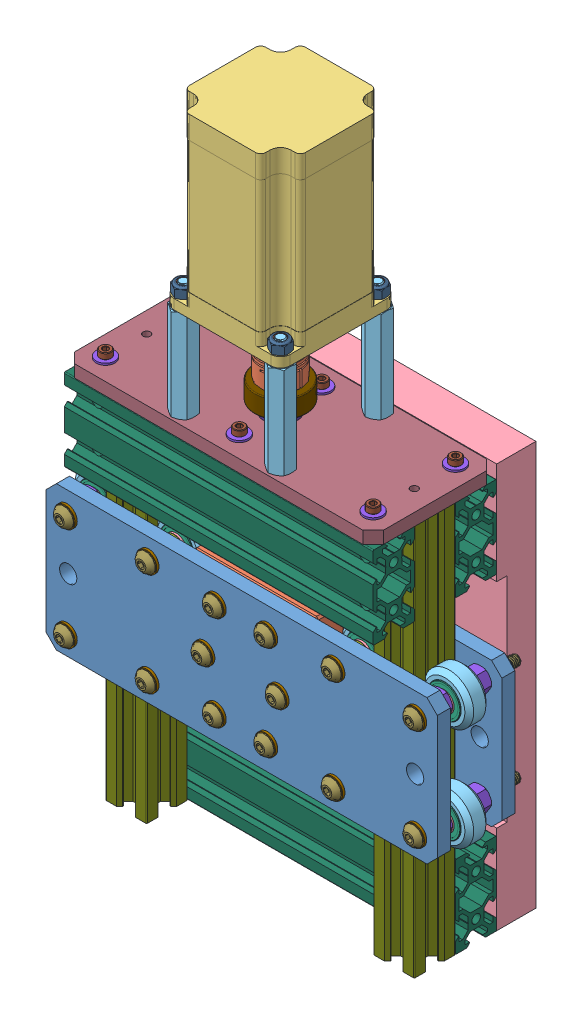
SolidWorks assembly Longitudinal Trim Assembly, configuration Default. Lengths in mm. (continued)
Components (placement in the parent): (continued)
- 91100A120 - WASHER, M3 X 9 OD, 18-8-2: 91100A120 - WASHER, M3 X 9 OD, 18-8 [93475A210] at (65 -65 17.3) x (0.993328 0.115328 0) z (0 0 1) size (9 9 0.9)
- 94500A222 - BHCS, M3-0.5 X 8, 316 SS-2: 94500A222 - BHCS, M3-0.5 X 8, 316 SS [94500A222] at (65 -65 15.65) x (-0.923728 -0.383049 0) z (0 0 -1) size (5.7 5.7 9.95)
- HNTTBS5-3 - NUT, PRE-INSERTION, M3 X 10 SQ, 18-8-3: HNTTBS5-3 - NUT, PRE-INSERTION, M3 X 10 SQ, 18-8 [Default] at (65 65 21.8) x (0 0 -1) z (0 -1 0) size (2.7 10 10)
- 91100A120 - WASHER, M3 X 9 OD, 18-8-3: 91100A120 - WASHER, M3 X 9 OD, 18-8 [93475A210] at (65 65 17.3) x (0.993328 0.115328 0) z (0 0 1) size (9 9 0.9)
- 94500A222 - BHCS, M3-0.5 X 8, 316 SS-3: 94500A222 - BHCS, M3-0.5 X 8, 316 SS [94500A222] at (65 65 15.65) x (-0.923728 -0.383049 0) z (0 0 -1) size (5.7 5.7 9.95)
- HNTTBS5-3 - NUT, PRE-INSERTION, M3 X 10 SQ, 18-8-4: HNTTBS5-3 - NUT, PRE-INSERTION, M3 X 10 SQ, 18-8 [Default] at (65 85 21.8) x (0 0 -1) z (0 -1 0) size (2.7 10 10)
- 91100A120 - WASHER, M3 X 9 OD, 18-8-4: 91100A120 - WASHER, M3 X 9 OD, 18-8 [93475A210] at (65 85 17.3) x (0.993328 0.115328 0) z (0 0 1) size (9 9 0.9)
- 94500A222 - BHCS, M3-0.5 X 8, 316 SS-4: 94500A222 - BHCS, M3-0.5 X 8, 316 SS [94500A222] at (65 85 15.65) x (-0.923728 -0.383049 0) z (0 0 -1) size (5.7 5.7 9.95)
- HNTTBS5-3 - NUT, PRE-INSERTION, M3 X 10 SQ, 18-8-5: HNTTBS5-3 - NUT, PRE-INSERTION, M3 X 10 SQ, 18-8 [Default] at (65 65 38.2) x (0 0 -1) z (0 -1 0) size (2.7 10 10)
- 91100A120 - WASHER, M3 X 9 OD, 18-8-5: 91100A120 - WASHER, M3 X 9 OD, 18-8 [93475A210] at (65 65 42.7) x (0.961741 0.273962 0) z (0 0 -1) size (9 9 0.9)
- 94500A222 - BHCS, M3-0.5 X 8, 316 SS-5: 94500A222 - BHCS, M3-0.5 X 8, 316 SS [94500A222] at (65 65 44.35) x (-0.923728 -0.383049 0) z (0 0 1) size (5.7 5.7 9.95)
- HNTTBS5-3 - NUT, PRE-INSERTION, M3 X 10 SQ, 18-8-6: HNTTBS5-3 - NUT, PRE-INSERTION, M3 X 10 SQ, 18-8 [Default] at (65 85 38.2) x (0 0 -1) z (0 -1 0) size (2.7 10 10)
- 91100A120 - WASHER, M3 X 9 OD, 18-8-6: 91100A120 - WASHER, M3 X 9 OD, 18-8 [93475A210] at (65 85 42.7) x (0.961741 0.273962 0) z (0 0 -1) size (9 9 0.9)
- 94500A222 - BHCS, M3-0.5 X 8, 316 SS-6: 94500A222 - BHCS, M3-0.5 X 8, 316 SS [94500A222] at (65 85 44.35) x (-1 0 0) z (0 0 1) size (5.7 5.7 9.95)
- HNTTBS5-3 - NUT, PRE-INSERTION, M3 X 10 SQ, 18-8-9: HNTTBS5-3 - NUT, PRE-INSERTION, M3 X 10 SQ, 18-8 [Default] at (-65 85 1.8) x (0 0 -1) z (1 0 0) size (2.7 10 10)
- 91420A130 - FHS, 90 DEG, M3-0.5 X 25, STEEL, ZINC-13: 91420A130 - FHS, 90 DEG, M3-0.5 X 25, STEEL, ZINC [91420A130] at (-65 85 -17.05) x (-0.923728 -0.383049 0) z (0 0 -1) size (5.6 5.6 25.28)
- HNTTBS5-3 - NUT, PRE-INSERTION, M3 X 10 SQ, 18-8-29: HNTTBS5-3 - NUT, PRE-INSERTION, M3 X 10 SQ, 18-8 [Default] at (65 93.2 50) x (0 1 0) z (1 0 0) size (2.7 10 10)
- 91100A120 - WASHER, M3 X 9 OD, 18-8-14: 91100A120 - WASHER, M3 X 9 OD, 18-8 [93475A210] at (65 101 50) x (0.993663 0 -0.112402) z (0 1 0) size (9 9 0.9)
- 91292A114 - SHCS, M3-0.5 X 12, 18-8-1: 91292A114 - SHCS, M3-0.5 X 12, 18-8 [91292A114] at (65 89.9 50) x (-0.862717 0 -0.505687) z (0 -1 0) size (5.5 5.5 15.23)
- HNTTBS5-3 - NUT, PRE-INSERTION, M3 X 10 SQ, 18-8-12: HNTTBS5-3 - NUT, PRE-INSERTION, M3 X 10 SQ, 18-8 [Default] at (0 -85 1.8) x (0 0 -1) z (1 0 0) size (2.7 10 10)
- HNTTBS5-3 - NUT, PRE-INSERTION, M3 X 10 SQ, 18-8-13: HNTTBS5-3 - NUT, PRE-INSERTION, M3 X 10 SQ, 18-8 [Default] at (0 -65 1.8) x (0 0 -1) z (1 0 0) size (2.7 10 10)
- HNTTBS5-3 - NUT, PRE-INSERTION, M3 X 10 SQ, 18-8-14: HNTTBS5-3 - NUT, PRE-INSERTION, M3 X 10 SQ, 18-8 [Default] at (0 65 1.8) x (0 0 -1) z (1 0 0) size (2.7 10 10)
- HNTTBS5-3 - NUT, PRE-INSERTION, M3 X 10 SQ, 18-8-15: HNTTBS5-3 - NUT, PRE-INSERTION, M3 X 10 SQ, 18-8 [Default] at (0 85 1.8) x (0 0 -1) z (1 0 0) size (2.7 10 10)
- HNTTBS5-3 - NUT, PRE-INSERTION, M3 X 10 SQ, 18-8-16: HNTTBS5-3 - NUT, PRE-INSERTION, M3 X 10 SQ, 18-8 [Default] at (-65 -85 1.8) x (0 0 -1) z (1 0 0) size (2.7 10 10)
- HNTTBS5-3 - NUT, PRE-INSERTION, M3 X 10 SQ, 18-8-17: HNTTBS5-3 - NUT, PRE-INSERTION, M3 X 10 SQ, 18-8 [Default] at (-65 -65 1.8) x (0 0 -1) z (1 0 0) size (2.7 10 10)
- HNTTBS5-3 - NUT, PRE-INSERTION, M3 X 10 SQ, 18-8-18: HNTTBS5-3 - NUT, PRE-INSERTION, M3 X 10 SQ, 18-8 [Default] at (65 -85 1.8) x (0 0 -1) z (1 0 0) size (2.7 10 10)
- HNTTBS5-3 - NUT, PRE-INSERTION, M3 X 10 SQ, 18-8-19: HNTTBS5-3 - NUT, PRE-INSERTION, M3 X 10 SQ, 18-8 [Default] at (-65 65 1.8) x (0 0 -1) z (1 0 0) size (2.7 10 10)
- HNTTBS5-3 - NUT, PRE-INSERTION, M3 X 10 SQ, 18-8-20: HNTTBS5-3 - NUT, PRE-INSERTION, M3 X 10 SQ, 18-8 [Default] at (65 65 1.8) x (0 0 -1) z (1 0 0) size (2.7 10 10)
- HNTTBS5-3 - NUT, PRE-INSERTION, M3 X 10 SQ, 18-8-21: HNTTBS5-3 - NUT, PRE-INSERTION, M3 X 10 SQ, 18-8 [Default] at (65 85 1.8) x (0 0 -1) z (1 0 0) size (2.7 10 10)
- HNTTBS5-3 - NUT, PRE-INSERTION, M3 X 10 SQ, 18-8-22: HNTTBS5-3 - NUT, PRE-INSERTION, M3 X 10 SQ, 18-8 [Default] at (65 -65 1.8) x (0 0 -1) z (1 0 0) size (2.7 10 10)
- 91420A130 - FHS, 90 DEG, M3-0.5 X 25, STEEL, ZINC-14: 91420A130 - FHS, 90 DEG, M3-0.5 X 25, STEEL, ZINC [91420A130] at (0 -85 -17.05) x (-0.923728 -0.383049 0) z (0 0 -1) size (5.6 5.6 25.28)
- 91420A130 - FHS, 90 DEG, M3-0.5 X 25, STEEL, ZINC-15: 91420A130 - FHS, 90 DEG, M3-0.5 X 25, STEEL, ZINC [91420A130] at (0 -65 -17.05) x (-0.923728 -0.383049 0) z (0 0 -1) size (5.6 5.6 25.28)
- 91420A130 - FHS, 90 DEG, M3-0.5 X 25, STEEL, ZINC-16: 91420A130 - FHS, 90 DEG, M3-0.5 X 25, STEEL, ZINC [91420A130] at (0 65 -17.05) x (-0.923728 -0.383049 0) z (0 0 -1) size (5.6 5.6 25.28)
- 91420A130 - FHS, 90 DEG, M3-0.5 X 25, STEEL, ZINC-17: 91420A130 - FHS, 90 DEG, M3-0.5 X 25, STEEL, ZINC [91420A130] at (0 85 -17.05) x (-0.923728 -0.383049 0) z (0 0 -1) size (5.6 5.6 25.28)
- 91420A130 - FHS, 90 DEG, M3-0.5 X 25, STEEL, ZINC-18: 91420A130 - FHS, 90 DEG, M3-0.5 X 25, STEEL, ZINC [91420A130] at (-65 -85 -17.05) x (-0.923728 -0.383049 0) z (0 0 -1) size (5.6 5.6 25.28)
- 91420A130 - FHS, 90 DEG, M3-0.5 X 25, STEEL, ZINC-19: 91420A130 - FHS, 90 DEG, M3-0.5 X 25, STEEL, ZINC [91420A130] at (-65 -65 -17.05) x (-0.923728 -0.383049 0) z (0 0 -1) size (5.6 5.6 25.28)
- 91420A130 - FHS, 90 DEG, M3-0.5 X 25, STEEL, ZINC-20: 91420A130 - FHS, 90 DEG, M3-0.5 X 25, STEEL, ZINC [91420A130] at (65 -85 -17.05) x (-0.923728 -0.383049 0) z (0 0 -1) size (5.6 5.6 25.28)
- 91420A130 - FHS, 90 DEG, M3-0.5 X 25, STEEL, ZINC-21: 91420A130 - FHS, 90 DEG, M3-0.5 X 25, STEEL, ZINC [91420A130] at (-65 65 -17.05) x (-0.923728 -0.383049 0) z (0 0 -1) size (5.6 5.6 25.28)
- 91420A130 - FHS, 90 DEG, M3-0.5 X 25, STEEL, ZINC-22: 91420A130 - FHS, 90 DEG, M3-0.5 X 25, STEEL, ZINC [91420A130] at (65 65 -17.05) x (-0.923728 -0.383049 0) z (0 0 -1) size (5.6 5.6 25.28)
- 91420A130 - FHS, 90 DEG, M3-0.5 X 25, STEEL, ZINC-23: 91420A130 - FHS, 90 DEG, M3-0.5 X 25, STEEL, ZINC [91420A130] at (65 85 -17.05) x (-0.923728 -0.383049 0) z (0 0 -1) size (5.6 5.6 25.28)
- 91420A130 - FHS, 90 DEG, M3-0.5 X 25, STEEL, ZINC-24: 91420A130 - FHS, 90 DEG, M3-0.5 X 25, STEEL, ZINC [91420A130] at (65 -65 -17.05) x (-0.923728 -0.383049 0) z (0 0 -1) size (5.6 5.6 25.28)
- HNTTBS5-3 - NUT, PRE-INSERTION, M3 X 10 SQ, 18-8-23: HNTTBS5-3 - NUT, PRE-INSERTION, M3 X 10 SQ, 18-8 [Default] at (-65 -85 21.8) x (0 0 -1) z (0 1 0) size (2.7 10 10)
- 91100A120 - WASHER, M3 X 9 OD, 18-8-8: 91100A120 - WASHER, M3 X 9 OD, 18-8 [93475A210] at (-65 -85 18.2) x (-0.993328 0.115328 0) z (0 0 -1) size (9 9 0.9)
- 94500A222 - BHCS, M3-0.5 X 8, 316 SS-8: 94500A222 - BHCS, M3-0.5 X 8, 316 SS [94500A222] at (-65 -85 15.65) x (0.923728 -0.383049 0) z (0 0 -1) size (5.7 5.7 9.95)
- HNTTBS5-3 - NUT, PRE-INSERTION, M3 X 10 SQ, 18-8-24: HNTTBS5-3 - NUT, PRE-INSERTION, M3 X 10 SQ, 18-8 [Default] at (-65 -65 21.8) x (0 0 -1) z (0 1 0) size (2.7 10 10)
- 91100A120 - WASHER, M3 X 9 OD, 18-8-9: 91100A120 - WASHER, M3 X 9 OD, 18-8 [93475A210] at (-65 -65 18.2) x (-0.993328 0.115328 0) z (0 0 -1) size (9 9 0.9)
- 94500A222 - BHCS, M3-0.5 X 8, 316 SS-9: 94500A222 - BHCS, M3-0.5 X 8, 316 SS [94500A222] at (-65 -65 15.65) x (0.923728 -0.383049 0) z (0 0 -1) size (5.7 5.7 9.95)
- HNTTBS5-3 - NUT, PRE-INSERTION, M3 X 10 SQ, 18-8-25: HNTTBS5-3 - NUT, PRE-INSERTION, M3 X 10 SQ, 18-8 [Default] at (-65 65 21.8) x (0 0 -1) z (0 1 0) size (2.7 10 10)
- 91100A120 - WASHER, M3 X 9 OD, 18-8-10: 91100A120 - WASHER, M3 X 9 OD, 18-8 [93475A210] at (-65 65 18.2) x (-0.993328 0.115328 0) z (0 0 -1) size (9 9 0.9)
- 94500A222 - BHCS, M3-0.5 X 8, 316 SS-10: 94500A222 - BHCS, M3-0.5 X 8, 316 SS [94500A222] at (-65 65 15.65) x (0.923728 -0.383049 0) z (0 0 -1) size (5.7 5.7 9.95)
- HNTTBS5-3 - NUT, PRE-INSERTION, M3 X 10 SQ, 18-8-26: HNTTBS5-3 - NUT, PRE-INSERTION, M3 X 10 SQ, 18-8 [Default] at (-65 85 21.8) x (0 0 -1) z (0 1 0) size (2.7 10 10)
- 91100A120 - WASHER, M3 X 9 OD, 18-8-11: 91100A120 - WASHER, M3 X 9 OD, 18-8 [93475A210] at (-65 85 18.2) x (-0.993328 0.115328 0) z (0 0 -1) size (9 9 0.9)
- 94500A222 - BHCS, M3-0.5 X 8, 316 SS-11: 94500A222 - BHCS, M3-0.5 X 8, 316 SS [94500A222] at (-65 85 15.65) x (0.923728 -0.383049 0) z (0 0 -1) size (5.7 5.7 9.95)
- HNTTBS5-3 - NUT, PRE-INSERTION, M3 X 10 SQ, 18-8-27: HNTTBS5-3 - NUT, PRE-INSERTION, M3 X 10 SQ, 18-8 [Default] at (-65 65 38.2) x (0 0 -1) z (0 1 0) size (2.7 10 10)
- 91100A120 - WASHER, M3 X 9 OD, 18-8-12: 91100A120 - WASHER, M3 X 9 OD, 18-8 [93475A210] at (-65 65 41.8) x (-0.961741 0.273962 0) z (0 0 1) size (9 9 0.9)
- 94500A222 - BHCS, M3-0.5 X 8, 316 SS-12: 94500A222 - BHCS, M3-0.5 X 8, 316 SS [94500A222] at (-65 65 44.35) x (0.923728 -0.383049 0) z (0 0 1) size (5.7 5.7 9.95)
- HNTTBS5-3 - NUT, PRE-INSERTION, M3 X 10 SQ, 18-8-28: HNTTBS5-3 - NUT, PRE-INSERTION, M3 X 10 SQ, 18-8 [Default] at (-65 85 38.2) x (0 0 -1) z (0 1 0) size (2.7 10 10)
- 91100A120 - WASHER, M3 X 9 OD, 18-8-13: 91100A120 - WASHER, M3 X 9 OD, 18-8 [93475A210] at (-65 85 41.8) x (-0.961741 0.273962 0) z (0 0 1) size (9 9 0.9)
- 94500A222 - BHCS, M3-0.5 X 8, 316 SS-13: 94500A222 - BHCS, M3-0.5 X 8, 316 SS [94500A222] at (-65 85 44.35) size (5.7 5.7 9.95)
- HNTTBS5-3 - NUT, PRE-INSERTION, M3 X 10 SQ, 18-8-31: HNTTBS5-3 - NUT, PRE-INSERTION, M3 X 10 SQ, 18-8 [Default] at (-65 93.2 10) x (0 1 0) z (1 0 0) size (2.7 10 10)
- HNTTBS5-3 - NUT, PRE-INSERTION, M3 X 10 SQ, 18-8-32: HNTTBS5-3 - NUT, PRE-INSERTION, M3 X 10 SQ, 18-8 [Default] at (65 93.2 10) x (0 1 0) z (1 0 0) size (2.7 10 10)
- HNTTBS5-3 - NUT, PRE-INSERTION, M3 X 10 SQ, 18-8-33: HNTTBS5-3 - NUT, PRE-INSERTION, M3 X 10 SQ, 18-8 [Default] at (0 93.2 50) x (0 1 0) z (1 0 0) size (2.7 10 10)
- HNTTBS5-3 - NUT, PRE-INSERTION, M3 X 10 SQ, 18-8-34: HNTTBS5-3 - NUT, PRE-INSERTION, M3 X 10 SQ, 18-8 [Default] at (0 93.2 10) x (0 1 0) z (1 0 0) size (2.7 10 10)
- HNTTBS5-3 - NUT, PRE-INSERTION, M3 X 10 SQ, 18-8-35: HNTTBS5-3 - NUT, PRE-INSERTION, M3 X 10 SQ, 18-8 [Default] at (-65 93.2 50) x (0 1 0) z (1 0 0) size (2.7 10 10)
- 91100A120 - WASHER, M3 X 9 OD, 18-8-15: 91100A120 - WASHER, M3 X 9 OD, 18-8 [93475A210] at (-65 101 10) x (0.993663 0 -0.112402) z (0 1 0) size (9 9 0.9)
- 91100A120 - WASHER, M3 X 9 OD, 18-8-16: 91100A120 - WASHER, M3 X 9 OD, 18-8 [93475A210] at (65 101 10) x (0.993663 0 -0.112402) z (0 1 0) size (9 9 0.9)
- 91100A120 - WASHER, M3 X 9 OD, 18-8-17: 91100A120 - WASHER, M3 X 9 OD, 18-8 [93475A210] at (0 101 50) x (0.993663 0 -0.112402) z (0 1 0) size (9 9 0.9)
- 91100A120 - WASHER, M3 X 9 OD, 18-8-18: 91100A120 - WASHER, M3 X 9 OD, 18-8 [93475A210] at (0 101 10) x (0.993663 0 -0.112402) z (0 1 0) size (9 9 0.9)
- 91100A120 - WASHER, M3 X 9 OD, 18-8-19: 91100A120 - WASHER, M3 X 9 OD, 18-8 [93475A210] at (-65 101 50) x (0.993663 0 -0.112402) z (0 1 0) size (9 9 0.9)
- 91292A114 - SHCS, M3-0.5 X 12, 18-8-2: 91292A114 - SHCS, M3-0.5 X 12, 18-8 [91292A114] at (-65 89.9 10) x (-0.862717 0 -0.505687) z (0 -1 0) size (5.5 5.5 15.23)
- 91292A114 - SHCS, M3-0.5 X 12, 18-8-3: 91292A114 - SHCS, M3-0.5 X 12, 18-8 [91292A114] at (65 89.9 10) x (-0.862717 0 -0.505687) z (0 -1 0) size (5.5 5.5 15.23)
- 91292A114 - SHCS, M3-0.5 X 12, 18-8-4: 91292A114 - SHCS, M3-0.5 X 12, 18-8 [91292A114] at (0 89.9 50) x (-0.862717 0 -0.505687) z (0 -1 0) size (5.5 5.5 15.23)
- 91292A114 - SHCS, M3-0.5 X 12, 18-8-5: 91292A114 - SHCS, M3-0.5 X 12, 18-8 [91292A114] at (0 89.9 10) x (-0.862717 0 -0.505687) z (0 -1 0) size (5.5 5.5 15.23)
- 91292A114 - SHCS, M3-0.5 X 12, 18-8-6: 91292A114 - SHCS, M3-0.5 X 12, 18-8 [91292A114] at (-65 89.9 50) x (-0.862717 0 -0.505687) z (0 -1 0) size (5.5 5.5 15.23)
Mates (geometry in assembly coordinates):
- Concentric56: concentric aligned: cylinder of MTSBRA12-160-S35-Q8-1 through (0 107.5 30) axis (0 -1 0) radius 4; cylinder of 819368020915 - Flexible Coupling 5mm x 0.25in-1 through (0 139.2137 30) axis (0 -1 0) radius 4
- Concentric57: concentric aligned: cylinder of 819368020915 - Flexible Coupling 5mm x 0.25in-1 through (0 127.9 30) axis (0 1 0) radius 3.175; cylinder of 819368021257 - Nema 23 High Torque Stepper Motor-1 through (0 125.4 30) axis (0 1 0) radius 3.175
- Parallel4: parallel aligned: plane of Rear Plate Assembly-1/Rear Plate-1 through (-75 95 60) normal (0 0 1); plane of 819368021257 - Nema 23 High Torque Stepper Motor-1 through (-23.6 150.8 58.2) normal (0 0 1)
- Coincident61: coincident anti-aligned: plane of 819368020915 - Flexible Coupling 5mm x 0.25in-1 through (0 140.4 30) normal (0 1 0); plane of 819368021257 - Nema 23 High Torque Stepper Motor-1 through (0 140.4 30) normal (0 -1 0)
- Distance2: distance = 45 mm anti-aligned: plane of 819368021257 - Nema 23 High Torque Stepper Motor-1 through (-23.6 146 53.6) normal (0 -1 0); plane of Rear Plate Assembly-1/Rear Plate-1 through (0 101 30) normal (0 1 0)
- Concentric58: concentric anti-aligned: cylinder of 819368021257 - Nema 23 High Torque Stepper Motor-1 through (-23.57 232.001 53.57) axis (0 -1 0) radius 2.55; cylinder of 94669A204 - SPACER, UNTHD, M5 X 13OD X 45L, 6061-T6-1 through (-23.57 101 53.57) axis (0 1 0) radius 2.65
- Coincident62: coincident anti-aligned: plane of 819368021257 - Nema 23 High Torque Stepper Motor-1 through (-23.6 146 53.6) normal (0 -1 0); plane of 94669A204 - SPACER, UNTHD, M5 X 13OD X 45L, 6061-T6-1 through (-23.57 146 53.57) normal (0 1 0)
- Concentric62: concentric aligned: cylinder of Rear Plate Assembly-1/Rear Plate-1 through (23.57 95 53.57) axis (0 -1 0) radius 2.9; circle of 93655A248 - STANDOFF, MALE-TO-FEMALE, M5-0.8 X 12.7 THD DPTH X 10 HEX X 45L, 18-8-1
- Coincident67: coincident anti-aligned: plane of Rear Plate Assembly-1/Rear Plate-1 through (0 101 30) normal (0 1 0); plane of 93655A248 - STANDOFF, MALE-TO-FEMALE, M5-0.8 X 12.7 THD DPTH X 10 HEX X 45L, 18-8-1 through (18.7366 101 50.4122) normal (0 -1 0)
- Concentric63: concentric anti-aligned: circle of 93655A248 - STANDOFF, MALE-TO-FEMALE, M5-0.8 X 12.7 THD DPTH X 10 HEX X 45L, 18-8-1; cylinder of 93475A240-17 through (23.57 151.9 53.57) axis (0 -1 0) radius 5
- Coincident68: coincident anti-aligned: plane of 819368021257 - Nema 23 High Torque Stepper Motor-1 through (-23.6 150.8 53.6) normal (0 1 0); plane of 93475A240-17 through (23.57 150.8 53.57) normal (0 -1 0)
- Concentric64: concentric anti-aligned: cylinder of 93475A240-17 through (23.57 151.9 53.57) axis (0 -1 0) radius 5; cylinder of 93625A200 - M5 x 0.8 mm Nylon-Insert Locknut-9/93625A200 - M5 x 0.8 mm Nylon-Insert Locknut_2-1 through (23.57 153.55 53.57) axis (0 1 0) radius 2.117
- Coincident69: coincident anti-aligned: plane of 93475A240-17 through (23.57 151.9 53.57) normal (0 1 0); plane of 93625A200 - M5 x 0.8 mm Nylon-Insert Locknut-9/93625A200 - M5 x 0.8 mm Nylon-Insert Locknut_2-1 through (27.4293 150.8 51.0324) normal (0 -1 0)
- Concentric65: concentric aligned: circle of 93655A248 - STANDOFF, MALE-TO-FEMALE, M5-0.8 X 12.7 THD DPTH X 10 HEX X 45L, 18-8-1; cylinder of 93625A200 - M5 x 0.8 mm Nylon-Insert Locknut-9/93625A200 - M5 x 0.8 mm Nylon-Insert Locknut_2-1 through (23.57 153.55 53.57) axis (0 1 0) radius 2.117
- Coincident70: coincident anti-aligned: plane of 819368021257 - Nema 23 High Torque Stepper Motor-1 through (-23.6 150.8 53.6) normal (0 1 0); plane of 93625A200 - M5 x 0.8 mm Nylon-Insert Locknut-9/93625A200 - M5 x 0.8 mm Nylon-Insert Locknut_2-1 through (27.4293 150.8 51.0324) normal (0 -1 0)
- Concentric66: concentric aligned: cone of Rear Plate Assembly-1/Rear Plate-1 through (23.57 95 53.57) axis (0 1 0); cone of 92125A107 - FHS, 90 DEG, M5-0.8 X 15, 18-8-1 through (23.57 98.7 53.57) axis (0 1 0)
- Coincident71: coincident aligned: cone of Rear Plate Assembly-1/Rear Plate-1 through (23.57 95 53.57) axis (0 1 0); cone of 92125A107 - FHS, 90 DEG, M5-0.8 X 15, 18-8-1 through (23.57 98.7 53.57) axis (0 1 0)
- Parallel5: parallel aligned: plane of Rear Plate Assembly-1/Rear Plate-1 through (-75 95 60) normal (0 0 1); plane of 819368020915 - Flexible Coupling 5mm x 0.25in-1 through (6.7 119.4 36.2) normal (0 0 1)
- Symmetric1: symmetric aligned: plane of Aft Frame Assembly-1/V-Slot 20x20x190 Linear Rail Tapped Ends-1 through (59.5 -405 30) normal (1 0 0); plane of HNTTBS5-3 - NUT, PRE-INSERTION, M3 X 10 SQ, 18-8-1 through (70.5 -405 30) normal (-1 0 0); plane of Aft Frame Assembly-1/V-Slot 20x20x190 Linear Rail Tapped Ends-1 through (65 -85 21.8) normal (1 0 0)
- Coincident88: coincident anti-aligned: plane of Aft Frame Assembly-1/V-Slot 20x20x190 Linear Rail Tapped Ends-1 through (65 -405 21.8) normal (0 0 1); plane of HNTTBS5-3 - NUT, PRE-INSERTION, M3 X 10 SQ, 18-8-1 through (60 -90 21.8) normal (0 0 -1)
- Concentric84: concentric anti-aligned: cylinder of V-Slot 20x40x150 Linear Rail-1 through (65 -85 10) axis (0 0 -1) radius 3; cylinder of HNTTBS5-3 - NUT, PRE-INSERTION, M3 X 10 SQ, 18-8-1 through (65 -85 21.8) axis (0 0 1) radius 1.2295
- Concentric85: concentric aligned: cone of HNTTBS5-3 - NUT, PRE-INSERTION, M3 X 10 SQ, 18-8-1 through (65 -85 24.5) axis (0 0 -1); cylinder of 91100A120 - WASHER, M3 X 9 OD, 18-8-1 through (65 -85 18.2) axis (0 0 -1) radius 4.5
- Coincident89: coincident anti-aligned: plane of V-Slot 20x40x150 Linear Rail-1 through (425 -75 18.2) normal (0 0 -1); plane of 91100A120 - WASHER, M3 X 9 OD, 18-8-1 through (65 -85 18.2) normal (0 0 1)
- Concentric86: concentric anti-aligned: cylinder of 91100A120 - WASHER, M3 X 9 OD, 18-8-1 through (65 -85 18.2) axis (0 0 -1) radius 4.5; circle of 94500A222 - BHCS, M3-0.5 X 8, 316 SS-1
- Coincident90: coincident anti-aligned: plane of 91100A120 - WASHER, M3 X 9 OD, 18-8-1 through (65 -85 17.3) normal (0 0 -1); plane of 94500A222 - BHCS, M3-0.5 X 8, 316 SS-1 through (66.0917 -87.6326 17.3) normal (0 0 1)
- Concentric87: concentric aligned: cone of HNTTBS5-3 - NUT, PRE-INSERTION, M3 X 10 SQ, 18-8-2 through (65 -65 24.5) axis (0 0 -1); cylinder of 91100A120 - WASHER, M3 X 9 OD, 18-8-2 through (65 -65 18.2) axis (0 0 -1) radius 4.5
- Concentric88: concentric anti-aligned: cylinder of 91100A120 - WASHER, M3 X 9 OD, 18-8-2 through (65 -65 18.2) axis (0 0 -1) radius 4.5; circle of 94500A222 - BHCS, M3-0.5 X 8, 316 SS-2
- Coincident91: coincident anti-aligned: plane of 91100A120 - WASHER, M3 X 9 OD, 18-8-2 through (65 -65 17.3) normal (0 0 -1); plane of 94500A222 - BHCS, M3-0.5 X 8, 316 SS-2 through (66.0917 -67.6326 17.3) normal (0 0 1)
- Symmetric2: symmetric aligned: plane of Aft Frame Assembly-1/V-Slot 20x20x190 Linear Rail Tapped Ends-1 through (59.5 -405 30) normal (1 0 0); plane of HNTTBS5-3 - NUT, PRE-INSERTION, M3 X 10 SQ, 18-8-2 through (70.5 -405 30) normal (-1 0 0); plane of Aft Frame Assembly-1/V-Slot 20x20x190 Linear Rail Tapped Ends-1 through (65 -65 21.8) normal (1 0 0)
- Coincident92: coincident anti-aligned: plane of Aft Frame Assembly-1/V-Slot 20x20x190 Linear Rail Tapped Ends-1 through (65 -405 21.8) normal (0 0 1); plane of HNTTBS5-3 - NUT, PRE-INSERTION, M3 X 10 SQ, 18-8-2 through (60 -70 21.8) normal (0 0 -1)
- Coincident93: coincident anti-aligned: plane of V-Slot 20x40x150 Linear Rail-1 through (425 -75 18.2) normal (0 0 -1); plane of 91100A120 - WASHER, M3 X 9 OD, 18-8-2 through (65 -65 18.2) normal (0 0 1)
- Concentric89: concentric anti-aligned: cylinder of V-Slot 20x40x150 Linear Rail-1 through (65 -65 10) axis (0 0 -1) radius 3; cylinder of HNTTBS5-3 - NUT, PRE-INSERTION, M3 X 10 SQ, 18-8-2 through (65 -65 21.8) axis (0 0 1) radius 1.2295
- Concentric90: concentric aligned: cone of HNTTBS5-3 - NUT, PRE-INSERTION, M3 X 10 SQ, 18-8-3 through (65 65 24.5) axis (0 0 -1); cylinder of 91100A120 - WASHER, M3 X 9 OD, 18-8-3 through (65 65 18.2) axis (0 0 -1) radius 4.5
- Concentric91: concentric anti-aligned: cylinder of 91100A120 - WASHER, M3 X 9 OD, 18-8-3 through (65 65 18.2) axis (0 0 -1) radius 4.5; circle of 94500A222 - BHCS, M3-0.5 X 8, 316 SS-3
- Coincident94: coincident anti-aligned: plane of 91100A120 - WASHER, M3 X 9 OD, 18-8-3 through (65 65 17.3) normal (0 0 -1); plane of 94500A222 - BHCS, M3-0.5 X 8, 316 SS-3 through (66.0917 62.3674 17.3) normal (0 0 1)
- Symmetric3: symmetric aligned: plane of Aft Frame Assembly-1/V-Slot 20x20x190 Linear Rail Tapped Ends-1 through (59.5 -405 30) normal (1 0 0); plane of HNTTBS5-3 - NUT, PRE-INSERTION, M3 X 10 SQ, 18-8-3 through (70.5 -405 30) normal (-1 0 0); plane of Aft Frame Assembly-1/V-Slot 20x20x190 Linear Rail Tapped Ends-1 through (65 65 21.8) normal (1 0 0)
- Coincident95: coincident anti-aligned: plane of Aft Frame Assembly-1/V-Slot 20x20x190 Linear Rail Tapped Ends-1 through (65 -405 21.8) normal (0 0 1); plane of HNTTBS5-3 - NUT, PRE-INSERTION, M3 X 10 SQ, 18-8-3 through (60 60 21.8) normal (0 0 -1)
- Coincident96: coincident anti-aligned: plane of V-Slot 20x40x150 Linear Rail-1 through (425 -75 18.2) normal (0 0 -1); plane of 91100A120 - WASHER, M3 X 9 OD, 18-8-3 through (65 65 18.2) normal (0 0 1)
- Concentric92: concentric anti-aligned: cylinder of Aft Frame Assembly-1/V-Slot 20x40x150 Linear Rail-1 through (65 65 10) axis (0 0 -1) radius 3; cylinder of HNTTBS5-3 - NUT, PRE-INSERTION, M3 X 10 SQ, 18-8-3 through (65 65 21.8) axis (0 0 1) radius 1.2295
- Concentric93: concentric aligned: cone of HNTTBS5-3 - NUT, PRE-INSERTION, M3 X 10 SQ, 18-8-4 through (65 85 24.5) axis (0 0 -1); cylinder of 91100A120 - WASHER, M3 X 9 OD, 18-8-4 through (65 85 18.2) axis (0 0 -1) radius 4.5
- Concentric94: concentric anti-aligned: cylinder of 91100A120 - WASHER, M3 X 9 OD, 18-8-4 through (65 85 18.2) axis (0 0 -1) radius 4.5; circle of 94500A222 - BHCS, M3-0.5 X 8, 316 SS-4
- Coincident97: coincident anti-aligned: plane of 91100A120 - WASHER, M3 X 9 OD, 18-8-4 through (65 85 17.3) normal (0 0 -1); plane of 94500A222 - BHCS, M3-0.5 X 8, 316 SS-4 through (66.0917 82.3674 17.3) normal (0 0 1)
- Symmetric4: symmetric aligned: plane of Aft Frame Assembly-1/V-Slot 20x20x190 Linear Rail Tapped Ends-1 through (59.5 -405 30) normal (1 0 0); plane of HNTTBS5-3 - NUT, PRE-INSERTION, M3 X 10 SQ, 18-8-4 through (70.5 -405 30) normal (-1 0 0); plane of Aft Frame Assembly-1/V-Slot 20x20x190 Linear Rail Tapped Ends-1 through (65 85 21.8) normal (1 0 0)
- Coincident98: coincident anti-aligned: plane of Aft Frame Assembly-1/V-Slot 20x20x190 Linear Rail Tapped Ends-1 through (65 -405 21.8) normal (0 0 1); plane of HNTTBS5-3 - NUT, PRE-INSERTION, M3 X 10 SQ, 18-8-4 through (60 80 21.8) normal (0 0 -1)
- Coincident99: coincident anti-aligned: plane of V-Slot 20x40x150 Linear Rail-1 through (425 -75 18.2) normal (0 0 -1); plane of 91100A120 - WASHER, M3 X 9 OD, 18-8-4 through (65 85 18.2) normal (0 0 1)
- Concentric95: concentric anti-aligned: cylinder of Aft Frame Assembly-1/V-Slot 20x40x150 Linear Rail-1 through (65 85 10) axis (0 0 -1) radius 3; cylinder of HNTTBS5-3 - NUT, PRE-INSERTION, M3 X 10 SQ, 18-8-4 through (65 85 21.8) axis (0 0 1) radius 1.2295
- Concentric96: concentric anti-aligned: cone of HNTTBS5-3 - NUT, PRE-INSERTION, M3 X 10 SQ, 18-8-5 through (65 65 40.9) axis (0 0 -1); cylinder of 91100A120 - WASHER, M3 X 9 OD, 18-8-5 through (65 65 41.8) axis (0 0 1) radius 4.5
- Concentric97: concentric anti-aligned: cylinder of 91100A120 - WASHER, M3 X 9 OD, 18-8-5 through (65 65 41.8) axis (0 0 1) radius 4.5; circle of 94500A222 - BHCS, M3-0.5 X 8, 316 SS-5
- Coincident100: coincident anti-aligned: plane of 91100A120 - WASHER, M3 X 9 OD, 18-8-5 through (65 65 42.7) normal (0 0 1); plane of 94500A222 - BHCS, M3-0.5 X 8, 316 SS-5 through (63.9083 67.6326 42.7) normal (0 0 -1)
- Symmetric5: symmetric aligned: plane of Aft Frame Assembly-1/V-Slot 20x20x190 Linear Rail Tapped Ends-1 through (59.5 -405 30) normal (1 0 0); plane of HNTTBS5-3 - NUT, PRE-INSERTION, M3 X 10 SQ, 18-8-5 through (70.5 -405 30) normal (-1 0 0); plane of Aft Frame Assembly-1/V-Slot 20x20x190 Linear Rail Tapped Ends-1 through (65 65 38.2) normal (1 0 0)
- Coincident103: coincident aligned: plane of Aft Frame Assembly-1/V-Slot 20x20x190 Linear Rail Tapped Ends-1 through (65 -405 38.2) normal (0 0 -1); plane of HNTTBS5-3 - NUT, PRE-INSERTION, M3 X 10 SQ, 18-8-5 through (60 60 38.2) normal (0 0 -1)
- Concentric98: concentric anti-aligned: cylinder of Aft Frame Assembly-1/V-Slot 20x40x150 Linear Rail-2 through (65 65 50) axis (0 0 -1) radius 3; cylinder of HNTTBS5-3 - NUT, PRE-INSERTION, M3 X 10 SQ, 18-8-5 through (65 65 38.2) axis (0 0 1) radius 1.2295
- Coincident104: coincident anti-aligned: plane of Aft Frame Assembly-1/V-Slot 20x40x150 Linear Rail-2 through (425 75 41.8) normal (0 0 1); plane of 91100A120 - WASHER, M3 X 9 OD, 18-8-5 through (65 65 41.8) normal (0 0 -1)
- Concentric99: concentric anti-aligned: cone of HNTTBS5-3 - NUT, PRE-INSERTION, M3 X 10 SQ, 18-8-6 through (65 85 40.9) axis (0 0 -1); cylinder of 91100A120 - WASHER, M3 X 9 OD, 18-8-6 through (65 85 41.8) axis (0 0 1) radius 4.5
- Concentric100: concentric anti-aligned: cylinder of 91100A120 - WASHER, M3 X 9 OD, 18-8-6 through (65 85 41.8) axis (0 0 1) radius 4.5; circle of 94500A222 - BHCS, M3-0.5 X 8, 316 SS-6
- Coincident105: coincident anti-aligned: plane of 91100A120 - WASHER, M3 X 9 OD, 18-8-6 through (65 85 42.7) normal (0 0 1); plane of 94500A222 - BHCS, M3-0.5 X 8, 316 SS-6 through (65 87.85 42.7) normal (0 0 -1)
- Symmetric6: symmetric aligned: plane of Aft Frame Assembly-1/V-Slot 20x20x190 Linear Rail Tapped Ends-1 through (59.5 -405 30) normal (1 0 0); plane of HNTTBS5-3 - NUT, PRE-INSERTION, M3 X 10 SQ, 18-8-6 through (70.5 -405 30) normal (-1 0 0); plane of Aft Frame Assembly-1/V-Slot 20x20x190 Linear Rail Tapped Ends-1 through (65 85 38.2) normal (1 0 0)
- Coincident106: coincident aligned: plane of Aft Frame Assembly-1/V-Slot 20x20x190 Linear Rail Tapped Ends-1 through (65 -405 38.2) normal (0 0 -1); plane of HNTTBS5-3 - NUT, PRE-INSERTION, M3 X 10 SQ, 18-8-6 through (60 80 38.2) normal (0 0 -1)
- Concentric101: concentric anti-aligned: cylinder of Aft Frame Assembly-1/V-Slot 20x40x150 Linear Rail-2 through (65 85 50) axis (0 0 -1) radius 3; cylinder of HNTTBS5-3 - NUT, PRE-INSERTION, M3 X 10 SQ, 18-8-6 through (65 85 38.2) axis (0 0 1) radius 1.2295
- Coincident107: coincident anti-aligned: plane of Aft Frame Assembly-1/V-Slot 20x40x150 Linear Rail-2 through (425 75 41.8) normal (0 0 1); plane of 91100A120 - WASHER, M3 X 9 OD, 18-8-6 through (65 85 41.8) normal (0 0 -1)
- Symmetric8: symmetric aligned: plane of Aft Frame Assembly-1/V-Slot 20x40x150 Linear Rail-1 through (425 90.5 10) normal (0 -1 0); plane of HNTTBS5-3 - NUT, PRE-INSERTION, M3 X 10 SQ, 18-8-9 through (425 79.5 10) normal (0 1 0); plane of Aft Frame Assembly-1/V-Slot 20x40x150 Linear Rail-1 through (-65 85 1.8) normal (0 1 0)
- Coincident109: coincident anti-aligned: plane of Aft Frame Assembly-1/V-Slot 20x40x150 Linear Rail-1 through (425 75 1.8) normal (0 0 1); plane of HNTTBS5-3 - NUT, PRE-INSERTION, M3 X 10 SQ, 18-8-9 through (-60 80 1.8) normal (0 0 -1)
- Concentric104: concentric anti-aligned: cylinder of Trim Riser Board-1 through (-65 85 -19.05) axis (0 0 -1) radius 1.8; cylinder of HNTTBS5-3 - NUT, PRE-INSERTION, M3 X 10 SQ, 18-8-9 through (-65 85 1.8) axis (0 0 1) radius 1.2295
- Concentric105: concentric anti-aligned: cone of HNTTBS5-3 - NUT, PRE-INSERTION, M3 X 10 SQ, 18-8-9 through (-65 85 4.5) axis (0 0 -1); circle of 91420A130 - FHS, 90 DEG, M3-0.5 X 25, STEEL, ZINC-1
- Coincident110: coincident aligned: cone of Trim Riser Board-1 through (-65 85 -19.05) axis (0 0 1); cone of 91420A130 - FHS, 90 DEG, M3-0.5 X 25, STEEL, ZINC-13 through (-65 85 -18.7) axis (0 0 1)
- Symmetric10: symmetric aligned: plane of Aft Frame Assembly-1/V-Slot 20x40x150 Linear Rail-2 through (425 75 55.5) normal (0 0 -1); plane of HNTTBS5-3 - NUT, PRE-INSERTION, M3 X 10 SQ, 18-8-29 through (425 75 44.5) normal (0 0 1); plane of Aft Frame Assembly-1/V-Slot 20x40x150 Linear Rail-2 through (65 93.2 50) normal (0 0 1)
- Coincident111: coincident anti-aligned: plane of Aft Frame Assembly-1/V-Slot 20x40x150 Linear Rail-2 through (425 93.2 50) normal (0 -1 0); plane of HNTTBS5-3 - NUT, PRE-INSERTION, M3 X 10 SQ, 18-8-29 through (70 93.2 45) normal (0 1 0)
- Concentric106: concentric anti-aligned: cylinder of Rear Plate Assembly-1/Rear Plate-1 through (65 101 50) axis (0 1 0) radius 1.8; cylinder of HNTTBS5-3 - NUT, PRE-INSERTION, M3 X 10 SQ, 18-8-29 through (65 93.2 50) axis (0 -1 0) radius 1.2295
- Concentric107: concentric aligned: cone of HNTTBS5-3 - NUT, PRE-INSERTION, M3 X 10 SQ, 18-8-29 through (65 92.9295 50) axis (0 -1 0); cylinder of 91100A120 - WASHER, M3 X 9 OD, 18-8-14 through (65 101.9 50) axis (0 -1 0) radius 4.5
- Coincident112: coincident anti-aligned: plane of Rear Plate Assembly-1/Rear Plate-1 through (0 101 30) normal (0 1 0); plane of 91100A120 - WASHER, M3 X 9 OD, 18-8-14 through (65 101 50) normal (0 -1 0)
- Concentric108: concentric aligned: cylinder of 91100A120 - WASHER, M3 X 9 OD, 18-8-14 through (65 101.9 50) axis (0 -1 0) radius 4.5; cylinder of 91292A114 - SHCS, M3-0.5 X 12, 18-8-1 through (65 104.9 50) axis (0 -1 0) radius 2.75
- Coincident113: coincident anti-aligned: plane of 91100A120 - WASHER, M3 X 9 OD, 18-8-14 through (65 101.9 50) normal (0 1 0); plane of 91292A114 - SHCS, M3-0.5 X 12, 18-8-1 through (65 101.9 50) normal (0 -1 0)
